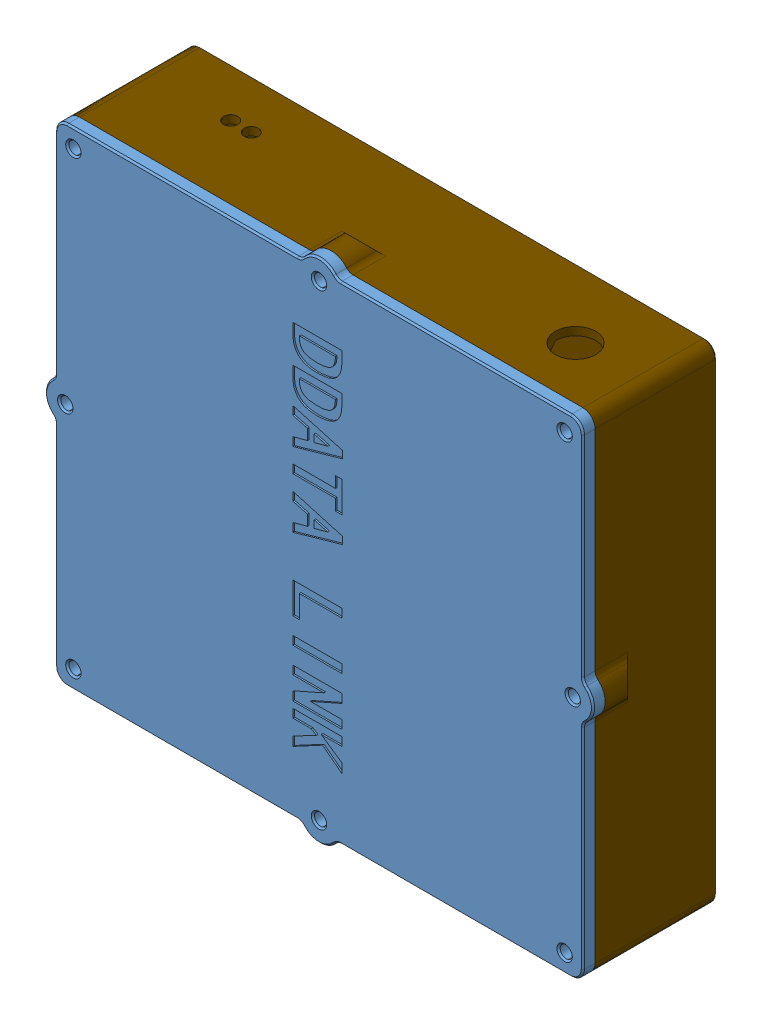
SolidWorks assembly 3D_DATA_LINK_2025-03-18, configuration 默认. Lengths in mm.
Overall size (135 126.5 33).
186 component instances, 20 part files, 8 mates.
Components (placement in the parent):
- 3D_DATA_LINK_2025-03-18.step-1: 3D_DATA_LINK_2025-03-18.step [默认] at (21.7099 -36.6353 -12.5128) size (99.97 88.97 17.5)
  - dtPB-USB5-HDR-TH_P2.54-V-M-R1-C2-S2.54.step-1: dtPB-USB5-HDR-TH_P2.54-V-M-R1-C2-S2.54.step [默认] at (28.7021 69.7231 1.6001) x (0 -1 0) z (0 0 1) size (2.54 5.09 11.5)
    - COMPOUND.step-1: COMPOUND.step [默认] at origin size (2.54 5.09 11.5)
  - dtPB-U3-SOT-23-5_L2.9-W1.6-P0.95-LS2.8-BR.step-1: dtPB-U3-SOT-23-5_L2.9-W1.6-P0.95-LS2.8-BR.step [默认] at (62.6111 64.0081 1.6001) x (-1 0 0) z (0 0 1) size (2.9 2.9 1.1)
    - COMPOUND-0.step-1: COMPOUND-0.step [默认] at origin size (2.9 2.9 1.1)
  - dtPB-I2-CONN-TH_3P-P2.54_2501S-3P.step-1: dtPB-I2-CONN-TH_3P-P2.54_2501S-3P.step [默认] at (107.6962 84.4963 1.6001) x (0 1 0) z (0 0 1) size (10 5.7 10.5)
    - COMPOUND-1.step-1: COMPOUND-1.step [默认] at origin size (10 5.7 10.5)
  - dtPB-I3-CONN-TH_3P-P2.54_2501S-3P.step-1: dtPB-I3-CONN-TH_3P-P2.54_2501S-3P.step [默认] at (100.2607 84.4963 1.6001) x (0 1 0) z (0 0 1) size (10 5.7 10.5)
    - COMPOUND-1.step-1: COMPOUND-1.step [默认] at origin size (10 5.7 10.5)
  - dtPB-I4-CONN-TH_3P-P2.54_2501S-3P.step-1: dtPB-I4-CONN-TH_3P-P2.54_2501S-3P.step [默认] at (92.8252 84.4963 1.6001) x (0 1 0) z (0 0 1) size (10 5.7 10.5)
    - COMPOUND-1.step-1: COMPOUND-1.step [默认] at origin size (10 5.7 10.5)
  - dtPB-I5-CONN-TH_3P-P2.54_2501S-3P.step-1: dtPB-I5-CONN-TH_3P-P2.54_2501S-3P.step [默认] at (85.3896 84.4963 1.6001) x (0 1 0) z (0 0 1) size (10 5.7 10.5)
    - COMPOUND-1.step-1: COMPOUND-1.step [默认] at origin size (10 5.7 10.5)
  - dtPB-I6-CONN-TH_3P-P2.54_2501S-3P.step-1: dtPB-I6-CONN-TH_3P-P2.54_2501S-3P.step [默认] at (63.083 84.4963 1.6001) x (0 1 0) z (0 0 1) size (10 5.7 10.5)
    - COMPOUND-1.step-1: COMPOUND-1.step [默认] at origin size (10 5.7 10.5)
  - dtPB-I7-CONN-TH_3P-P2.54_2501S-3P.step-1: dtPB-I7-CONN-TH_3P-P2.54_2501S-3P.step [默认] at (55.6475 84.4963 1.6001) x (0 1 0) z (0 0 1) size (10 5.7 10.5)
    - COMPOUND-1.step-1: COMPOUND-1.step [默认] at origin size (10 5.7 10.5)
  - dtPB-O1-CONN-TH_3P-P2.54_2501S-3P.step-1: dtPB-O1-CONN-TH_3P-P2.54_2501S-3P.step [默认] at (15.7076 34.7933 1.6001) x (-1 0 0) z (0 0 1) size (10 5.7 10.5)
    - COMPOUND-1.step-1: COMPOUND-1.step [默认] at origin size (10 5.7 10.5)
  - dtPB-O2-CONN-TH_3P-P2.54_2501S-3P.step-1: dtPB-O2-CONN-TH_3P-P2.54_2501S-3P.step [默认] at (15.7076 27.2931 1.6001) x (-1 0 0) z (0 0 1) size (10 5.7 10.5)
    - COMPOUND-1.step-1: COMPOUND-1.step [默认] at origin size (10 5.7 10.5)
  - dtPB-O3-CONN-TH_3P-P2.54_2501S-3P.step-1: dtPB-O3-CONN-TH_3P-P2.54_2501S-3P.step [默认] at (15.621 11.938 1.6001) x (-1 0 0) z (0 0 1) size (10 5.7 10.5)
    - COMPOUND-1.step-1: COMPOUND-1.step [默认] at origin size (10 5.7 10.5)
  - dtPB-O4-CONN-TH_3P-P2.54_2501S-3P.step-1: dtPB-O4-CONN-TH_3P-P2.54_2501S-3P.step [默认] at (15.7076 4.318 1.6001) x (-1 0 0) z (0 0 1) size (10 5.7 10.5)
    - COMPOUND-1.step-1: COMPOUND-1.step [默认] at origin size (10 5.7 10.5)
  - dtPB-O5-CONN-TH_3P-P2.54_2501S-3P.step-1: dtPB-O5-CONN-TH_3P-P2.54_2501S-3P.step [默认] at (26.7971 5.842 1.6001) x (0 -1 0) z (0 0 1) size (10 5.7 10.5)
    - COMPOUND-1.step-1: COMPOUND-1.step [默认] at origin size (10 5.7 10.5)
  - dtPB-O6-CONN-TH_3P-P2.54_2501S-3P.step-1: dtPB-O6-CONN-TH_3P-P2.54_2501S-3P.step [默认] at (34.1313 5.842 1.6001) x (0 -1 0) z (0 0 1) size (10 5.7 10.5)
    - COMPOUND-1.step-1: COMPOUND-1.step [默认] at origin size (10 5.7 10.5)
  - dtPB-O7-CONN-TH_3P-P2.54_2501S-3P.step-1: dtPB-O7-CONN-TH_3P-P2.54_2501S-3P.step [默认] at (41.4656 5.842 1.6001) x (0 -1 0) z (0 0 1) size (10 5.7 10.5)
    - COMPOUND-1.step-1: COMPOUND-1.step [默认] at origin size (10 5.7 10.5)
  - dtPB-PT100-CONN-TH_3P-P2.54_2501S-3P.step-1: dtPB-PT100-CONN-TH_3P-P2.54_2501S-3P.step [默认] at (78.1369 5.842 1.6001) x (0 -1 0) z (0 0 1) size (10 5.7 10.5)
    - COMPOUND-1.step-1: COMPOUND-1.step [默认] at origin size (10 5.7 10.5)
  - dtPB-PT101-CONN-TH_3P-P2.54_2501S-3P.step-1: dtPB-PT101-CONN-TH_3P-P2.54_2501S-3P.step [默认] at (85.4712 5.842 1.6001) x (0 -1 0) z (0 0 1) size (10 5.7 10.5)
    - COMPOUND-1.step-1: COMPOUND-1.step [默认] at origin size (10 5.7 10.5)
  - dtPB-PT102-CONN-TH_3P-P2.54_2501S-3P.step-1: dtPB-PT102-CONN-TH_3P-P2.54_2501S-3P.step [默认] at (105.1963 3.302 1.6001) size (10 5.7 10.5)
    - COMPOUND-1.step-1: COMPOUND-1.step [默认] at origin size (10 5.7 10.5)
  - dtPB-PT103-CONN-TH_3P-P2.54_2501S-3P.step-1: dtPB-PT103-CONN-TH_3P-P2.54_2501S-3P.step [默认] at (105.1963 11.2713 1.6001) size (10 5.7 10.5)
    - COMPOUND-1.step-1: COMPOUND-1.step [默认] at origin size (10 5.7 10.5)
  - dtPB-PWM1-CONN-TH_3P-P2.54_2501S-3P.step-1: dtPB-PWM1-CONN-TH_3P-P2.54_2501S-3P.step [默认] at (15.7076 50.0477 1.6001) x (-1 0 0) z (0 0 1) size (10 5.7 10.5)
    - COMPOUND-1.step-1: COMPOUND-1.step [默认] at origin size (10 5.7 10.5)
  - dtPB-PWM2-CONN-TH_3P-P2.54_2501S-3P.step-1: dtPB-PWM2-CONN-TH_3P-P2.54_2501S-3P.step [默认] at (15.7076 42.4205 1.6001) x (-1 0 0) z (0 0 1) size (10 5.7 10.5)
    - COMPOUND-1.step-1: COMPOUND-1.step [默认] at origin size (10 5.7 10.5)
  - dtPB-PWM3-CONN-TH_3P-P2.54_2501S-3P.step-1: dtPB-PWM3-CONN-TH_3P-P2.54_2501S-3P.step [默认] at (105.1963 59.0869 1.6001) size (10 5.7 10.5)
    - COMPOUND-1.step-1: COMPOUND-1.step [默认] at origin size (10 5.7 10.5)
  - dtPB-PWM4-CONN-TH_3P-P2.54_2501S-3P.step-1: dtPB-PWM4-CONN-TH_3P-P2.54_2501S-3P.step [默认] at (105.1963 67.0561 1.6001) size (10 5.7 10.5)
    - COMPOUND-1.step-1: COMPOUND-1.step [默认] at origin size (10 5.7 10.5)
  - dtPB-PWM5-CONN-TH_3P-P2.54_2501S-3P.step-1: dtPB-PWM5-CONN-TH_3P-P2.54_2501S-3P.step [默认] at (77.9541 84.4963 1.6001) x (0 1 0) z (0 0 1) size (10 5.7 10.5)
    - COMPOUND-1.step-1: COMPOUND-1.step [默认] at origin size (10 5.7 10.5)
  - dtPB-PWM6-CONN-TH_3P-P2.54_2501S-3P.step-1: dtPB-PWM6-CONN-TH_3P-P2.54_2501S-3P.step [默认] at (70.5186 84.4963 1.6001) x (0 1 0) z (0 0 1) size (10 5.7 10.5)
    - COMPOUND-1.step-1: COMPOUND-1.step [默认] at origin size (10 5.7 10.5)
  - dtPB-CURRENT1-CONN-TH_3P-P2.54_2501S-3P.step-1: dtPB-CURRENT1-CONN-TH_3P-P2.54_2501S-3P.step [默认] at (63.4684 5.842 1.6001) x (0 -1 0) z (0 0 1) size (10 5.7 10.5)
    - COMPOUND-1.step-1: COMPOUND-1.step [默认] at origin size (10 5.7 10.5)
  - dtPB-CURRENT2-CONN-TH_3P-P2.54_2501S-3P.step-1: dtPB-CURRENT2-CONN-TH_3P-P2.54_2501S-3P.step [默认] at (70.8026 5.842 1.6001) x (0 -1 0) z (0 0 1) size (10 5.7 10.5)
    - COMPOUND-1.step-1: COMPOUND-1.step [默认] at origin size (10 5.7 10.5)
  - dtPB-CURRENT3-CONN-TH_3P-P2.54_2501S-3P.step-1: dtPB-CURRENT3-CONN-TH_3P-P2.54_2501S-3P.step [默认] at (105.1963 19.2405 1.6001) size (10 5.7 10.5)
    - COMPOUND-1.step-1: COMPOUND-1.step [默认] at origin size (10 5.7 10.5)
  - dtPB-CURRENT4-CONN-TH_3P-P2.54_2501S-3P.step-1: dtPB-CURRENT4-CONN-TH_3P-P2.54_2501S-3P.step [默认] at (105.1963 27.2098 1.6001) size (10 5.7 10.5)
    - COMPOUND-1.step-1: COMPOUND-1.step [默认] at origin size (10 5.7 10.5)
  - dtPB-FLOW1-CONN-TH_3P-P2.54_2501S-3P.step-1: dtPB-FLOW1-CONN-TH_3P-P2.54_2501S-3P.step [默认] at (105.1963 35.1791 1.6001) size (10 5.7 10.5)
    - COMPOUND-1.step-1: COMPOUND-1.step [默认] at origin size (10 5.7 10.5)
  - dtPB-FLOW2-CONN-TH_3P-P2.54_2501S-3P.step-1: dtPB-FLOW2-CONN-TH_3P-P2.54_2501S-3P.step [默认] at (105.1963 43.1483 1.6001) size (10 5.7 10.5)
    - COMPOUND-1.step-1: COMPOUND-1.step [默认] at origin size (10 5.7 10.5)
  - dtPB-FLOW3-CONN-TH_3P-P2.54_2501S-3P.step-1: dtPB-FLOW3-CONN-TH_3P-P2.54_2501S-3P.step [默认] at (48.7998 5.842 1.6001) x (0 -1 0) z (0 0 1) size (10 5.7 10.5)
    - COMPOUND-1.step-1: COMPOUND-1.step [默认] at origin size (10 5.7 10.5)
  - dtPB-FLOW4-CONN-TH_3P-P2.54_2501S-3P.step-1: dtPB-FLOW4-CONN-TH_3P-P2.54_2501S-3P.step [默认] at (56.1341 5.842 1.6001) x (0 -1 0) z (0 0 1) size (10 5.7 10.5)
    - COMPOUND-1.step-1: COMPOUND-1.step [默认] at origin size (10 5.7 10.5)
  - dtPB-I1-CONN-TH_3P-P2.54_2501S-3P.step-1: dtPB-I1-CONN-TH_3P-P2.54_2501S-3P.step [默认] at (105.1963 51.1176 1.6001) size (10 5.7 10.5)
    - COMPOUND-1.step-1: COMPOUND-1.step [默认] at origin size (10 5.7 10.5)
  - dtPB-R2-R0603.step-1: dtPB-R2-R0603.step [默认] at (41.0617 61.009 1.6001) x (0 1 0) z (0 0 1) size (1.62 0.81 0.45)
    - COMPOUND-2.step-1: COMPOUND-2.step [默认] at origin size (1.62 0.81 0.45)
  - dtPB-R3-R0603.step-1: dtPB-R3-R0603.step [默认] at (41.0211 57.4041 1.6001) x (0 1 0) z (0 0 1) size (1.62 0.81 0.45)
    - COMPOUND-2.step-1: COMPOUND-2.step [默认] at origin size (1.62 0.81 0.45)
  - dtPB-R4-R0603.step-1: dtPB-R4-R0603.step [默认] at (40.0051 53.5941 1.6001) x (-1 0 0) z (0 0 1) size (1.62 0.81 0.45)
    - COMPOUND-2.step-1: COMPOUND-2.step [默认] at origin size (1.62 0.81 0.45)
  - dtPB-R5-R0603.step-1: dtPB-R5-R0603.step [默认] at (36.7031 53.5941 1.6001) x (-1 0 0) z (0 0 1) size (1.62 0.81 0.45)
    - COMPOUND-2.step-1: COMPOUND-2.step [默认] at origin size (1.62 0.81 0.45)
  - dtPB-R6-R0603.step-1: dtPB-R6-R0603.step [默认] at (60.8331 29.3371 1.6001) x (0 1 0) z (0 0 1) size (1.62 0.81 0.45)
    - COMPOUND-2.step-1: COMPOUND-2.step [默认] at origin size (1.62 0.81 0.45)
  - dtPB-R7-R0603.step-1: dtPB-R7-R0603.step [默认] at (33.1471 71.5011 1.6001) size (1.62 0.81 0.45)
    - COMPOUND-2.step-1: COMPOUND-2.step [默认] at origin size (1.62 0.81 0.45)
  - dtPB-R8-R0603.step-1: dtPB-R8-R0603.step [默认] at (58.5471 39.6241 1.6001) x (-1 0 0) z (0 0 1) size (1.62 0.81 0.45)
    - COMPOUND-2.step-1: COMPOUND-2.step [默认] at origin size (1.62 0.81 0.45)
  - dtPB-R9-R0603.step-1: dtPB-R9-R0603.step [默认] at (69.5961 29.5911 1.6001) x (0 1 0) z (0 0 1) size (1.62 0.81 0.45)
    - COMPOUND-2.step-1: COMPOUND-2.step [默认] at origin size (1.62 0.81 0.45)
  - dtPB-R18-R0603.step-1: dtPB-R18-R0603.step [默认] at (98.9529 37.3381 1.6001) x (0 -1 0) z (0 0 1) size (1.62 0.81 0.45)
    - COMPOUND-2.step-1: COMPOUND-2.step [默认] at origin size (1.62 0.81 0.45)
  - dtPB-R19-R0603.step-1: dtPB-R19-R0603.step [默认] at (98.9529 45.3724 1.6001) x (0 -1 0) z (0 0 1) size (1.62 0.81 0.45)
    - COMPOUND-2.step-1: COMPOUND-2.step [默认] at origin size (1.62 0.81 0.45)
  - dtPB-R20-R0603.step-1: dtPB-R20-R0603.step [默认] at (51.0541 12.3458 1.6001) x (-1 0 0) z (0 0 1) size (1.62 0.81 0.45)
    - COMPOUND-2.step-1: COMPOUND-2.step [默认] at origin size (1.62 0.81 0.45)
  - dtPB-R21-R0603.step-1: dtPB-R21-R0603.step [默认] at (58.4508 12.4728 1.6001) x (-1 0 0) z (0 0 1) size (1.62 0.81 0.45)
    - COMPOUND-2.step-1: COMPOUND-2.step [默认] at origin size (1.62 0.81 0.45)
  - dtPB-R22-R0603.step-1: dtPB-R22-R0603.step [默认] at (62.2301 12.4728 1.6001) size (1.62 0.81 0.45)
    - COMPOUND-2.step-1: COMPOUND-2.step [默认] at origin size (1.62 0.81 0.45)
  - dtPB-R23-R0603.step-1: dtPB-R23-R0603.step [默认] at (69.5961 12.3458 1.6001) size (1.62 0.81 0.45)
    - COMPOUND-2.step-1: COMPOUND-2.step [默认] at origin size (1.62 0.81 0.45)
  - dtPB-R24-R0603.step-1: dtPB-R24-R0603.step [默认] at (98.8062 18.161 1.6001) x (0 1 0) z (0 0 1) size (1.62 0.81 0.45)
    - COMPOUND-2.step-1: COMPOUND-2.step [默认] at origin size (1.62 0.81 0.45)
  - dtPB-R25-R0603.step-1: dtPB-R25-R0603.step [默认] at (98.8259 25.7811 1.6001) x (0 1 0) z (0 0 1) size (1.62 0.81 0.45)
    - COMPOUND-2.step-1: COMPOUND-2.step [默认] at origin size (1.62 0.81 0.45)
  - dtPB-R26-R0603.step-1: dtPB-R26-R0603.step [默认] at (76.8969 12.4217 1.6001) size (1.62 0.81 0.45)
    - COMPOUND-2.step-1: COMPOUND-2.step [默认] at origin size (1.62 0.81 0.45)
  - dtPB-R27-R0603.step-1: dtPB-R27-R0603.step [默认] at (80.3912 12.446 1.6001) x (-1 0 0) z (0 0 1) size (1.62 0.81 0.45)
    - COMPOUND-2.step-1: COMPOUND-2.step [默认] at origin size (1.62 0.81 0.45)
  - dtPB-R28-R0603.step-1: dtPB-R28-R0603.step [默认] at (97.9172 2.54 1.6001) x (0 1 0) z (0 0 1) size (1.62 0.81 0.45)
    - COMPOUND-2.step-1: COMPOUND-2.step [默认] at origin size (1.62 0.81 0.45)
  - dtPB-R29-R0603.step-1: dtPB-R29-R0603.step [默认] at (97.9172 5.969 1.6001) x (0 -1 0) z (0 0 1) size (1.62 0.81 0.45)
    - COMPOUND-2.step-1: COMPOUND-2.step [默认] at origin size (1.62 0.81 0.45)
  - dtPB-R30-R0603.step-1: dtPB-R30-R0603.step [默认] at (97.9172 10.16 1.6001) x (0 1 0) z (0 0 1) size (1.62 0.81 0.45)
    - COMPOUND-2.step-1: COMPOUND-2.step [默认] at origin size (1.62 0.81 0.45)
  - dtPB-R31-R0603.step-1: dtPB-R31-R0603.step [默认] at (97.9725 13.4275 1.6001) x (0 -1 0) z (0 0 1) size (1.62 0.81 0.45)
    - COMPOUND-2.step-1: COMPOUND-2.step [默认] at origin size (1.62 0.81 0.45)
  - dtPB-R32-R0603.step-1: dtPB-R32-R0603.step [默认] at (84.2565 12.4217 1.6001) size (1.62 0.81 0.45)
    - COMPOUND-2.step-1: COMPOUND-2.step [默认] at origin size (1.62 0.81 0.45)
  - dtPB-R33-R0603.step-1: dtPB-R33-R0603.step [默认] at (87.6855 12.4217 1.6001) x (-1 0 0) z (0 0 1) size (1.62 0.81 0.45)
    - COMPOUND-2.step-1: COMPOUND-2.step [默认] at origin size (1.62 0.81 0.45)
  - dtPB-R1-R0603.step-1: dtPB-R1-R0603.step [默认] at (41.0211 64.5161 1.6001) x (0 1 0) z (0 0 1) size (1.62 0.81 0.45)
    - COMPOUND-2.step-1: COMPOUND-2.step [默认] at origin size (1.62 0.81 0.45)
  - dtPB-IC1-CONN-TH_4P-P2.50_4PIN.step-1: dtPB-IC1-CONN-TH_4P-P2.50_4PIN.step [默认] at (16.891 19.558 1.6001) x (-1 0 0) z (0 0 1) size (12.5 5.7 10)
    - COMPOUND-3.step-1: COMPOUND-3.step [默认] at origin size (12.5 5.7 10)
  - dtPB-USART1-CONN-TH_4P-P2.50_4PIN.step-1: dtPB-USART1-CONN-TH_4P-P2.50_4PIN.step [默认] at (48.0061 83.2532 1.6001) x (0 1 0) z (0 0 1) size (12.5 5.7 10)
    - COMPOUND-3.step-1: COMPOUND-3.step [默认] at origin size (12.5 5.7 10)
  - dtPB-DOWNLOAD1-CONN-TH_4P-P2.50_4PIN.step-1: dtPB-DOWNLOAD1-CONN-TH_4P-P2.50_4PIN.step [默认] at (16.891 57.9121 1.6001) x (-1 0 0) z (0 0 1) size (12.5 5.7 10)
    - COMPOUND-3.step-1: COMPOUND-3.step [默认] at origin size (12.5 5.7 10)
  - dtPB-U5-WIRELM-SMD_E43-433T13S3.step-1: dtPB-U5-WIRELM-SMD_E43-433T13S3.step [默认] at (35.0521 31.2421 1.6001) x (-1 0 0) z (0 0 1) size (16 26 3.23)
    - COMPOUND-4.step-1: COMPOUND-4.step [默认] at origin size (16 26 3.23)
  - dtPB-VCC1-CONN-TH_2P-P5.00_WJ500V-5.08-2P.step-1: dtPB-VCC1-CONN-TH_2P-P5.00_WJ500V-5.08-2P.step [默认] at (20.32 83.8202 1.6001) size (10.76 10 17.5)
    - COMPOUND-5.step-1: COMPOUND-5.step [默认] at origin size (10.76 10 17.5)
  - dtPB-V5-CONN-TH_2P-P2.50_HX25003-2A.step-1: dtPB-V5-CONN-TH_2P-P2.50_HX25003-2A.step [默认] at (14.351 66.0401 1.6001) size (7.5 5.9 10.6)
    - COMPOUND-6.step-1: COMPOUND-6.step [默认] at origin size (7.5 5.9 10.6)
  - dtPB-U2-SOT-23-6_L2.9-W1.6-P0.95-LS2.8-BL.step-1: dtPB-U2-SOT-23-6_L2.9-W1.6-P0.95-LS2.8-BL.step [默认] at (36.4491 56.7691 1.6001) x (0 -1 0) z (0 0 1) size (2.88 2.79 1.64)
    - COMPOUND-7.step-1: COMPOUND-7.step [默认] at origin size (2.88 2.79 1.64)
  - dtPB-U1-LQFP-64_L10.0-W10.0-P0.50-LS12.0-BL.step-1: dtPB-U1-LQFP-64_L10.0-W10.0-P0.50-LS12.0-BL.step [默认] at (70.3581 41.6561 1.6001) size (12 12 1.45)
    - COMPOUND-8.step-1: COMPOUND-8.step [默认] at origin size (12 12 1.45)
  - dtPB-Board.step-1: dtPB-Board.step [默认] at origin size (99.97 88.97 1.6)
  - dtPB-C137-CAP-SMD_BD6.3-L6.6-W6.6-LS7.6-FD-1.step-1: dtPB-C137-CAP-SMD_BD6.3-L6.6-W6.6-LS7.6-FD-1.step [默认] at (20.447 73.1521 1.6001) size (7.2 6.6 7.72)
  - dtPB-C137-CAP-SMD_BD6.3-L6.6-W6.6-LS7.6-FD-1.step-2: dtPB-C137-CAP-SMD_BD6.3-L6.6-W6.6-LS7.6-FD-1.step [默认] at (49.9111 60.8331 1.6001) x (0 -1 0) z (0 0 1) size (7.2 6.6 7.72)
  - dtPB-C1-C0805.step-1: dtPB-C1-C0805.step [默认] at (35.9411 64.0081 1.6001) x (0 1 0) z (0 0 1) size (2 1.3 1.3)
  - dtPB-C1-C0805.step-2: dtPB-C1-C0805.step [默认] at (38.4811 64.0081 1.6001) x (0 1 0) z (0 0 1) size (2 1.3 1.3)
  - dtPB-C1-C0805.step-3: dtPB-C1-C0805.step [默认] at (49.5301 42.5451 1.6001) x (0 -1 0) z (0 0 1) size (2 1.3 1.3)
  - dtPB-C1-C0805.step-4: dtPB-C1-C0805.step [默认] at (30.3531 55.3721 1.6001) x (0 -1 0) z (0 0 1) size (2 1.3 1.3)
  - dtPB-C2-C0603.step-1: dtPB-C2-C0603.step [默认] at (43.1801 60.9601 1.6001) x (0 1 0) z (0 0 1) size (1.6 0.8 0.8)
  - dtPB-C2-C0603.step-2: dtPB-C2-C0603.step [默认] at (36.1951 60.1981 1.6001) x (-1 0 0) z (0 0 1) size (1.6 0.8 0.8)
  - dtPB-C2-C0603.step-3: dtPB-C2-C0603.step [默认] at (59.0551 64.2621 1.6001) x (0 1 0) z (0 0 1) size (1.6 0.8 0.8)
  - dtPB-C2-C0603.step-4: dtPB-C2-C0603.step [默认] at (65.9131 64.1351 1.6001) x (0 1 0) z (0 0 1) size (1.6 0.8 0.8)
  - dtPB-C2-C0603.step-5: dtPB-C2-C0603.step [默认] at (58.5471 37.5921 1.6001) size (1.6 0.8 0.8)
  - dtPB-C2-C0603.step-6: dtPB-C2-C0603.step [默认] at (73.716 29.5848 1.6001) x (0 1 0) z (0 0 1) size (1.6 0.8 0.8)
  - dtPB-C2-C0603.step-7: dtPB-C2-C0603.step [默认] at (84.5822 38.8621 1.6001) size (1.6 0.8 0.8)
  - dtPB-C2-C0603.step-8: dtPB-C2-C0603.step [默认] at (66.5481 55.2451 1.6001) x (0 -1 0) z (0 0 1) size (1.6 0.8 0.8)
  - dtPB-C2-C0603.step-9: dtPB-C2-C0603.step [默认] at (84.5822 45.7201 1.6001) size (1.6 0.8 0.8)
  - dtPB-C2-C0603.step-10: dtPB-C2-C0603.step [默认] at (63.8896 25.3945 1.6001) x (0 1 0) z (0 0 1) size (1.6 0.8 0.8)
  - dtPB-C2-C0603.step-11: dtPB-C2-C0603.step [默认] at (66.1671 25.4001 1.6001) x (0 1 0) z (0 0 1) size (1.6 0.8 0.8)
  - dtPB-C2-C0603.step-12: dtPB-C2-C0603.step [默认] at (71.3741 29.5911 1.6001) x (0 -1 0) z (0 0 1) size (1.6 0.8 0.8)
  - dtPB-C2-C0603.step-13: dtPB-C2-C0603.step [默认] at (46.7361 42.0371 1.6001) x (0 -1 0) z (0 0 1) size (1.6 0.8 0.8)
  - dtPB-C2-C0603.step-14: dtPB-C2-C0603.step [默认] at (77.0231 14.8655 1.6001) size (1.6 0.8 0.8)
  - dtPB-C2-C0603.step-15: dtPB-C2-C0603.step [默认] at (80.4521 14.8655 1.6001) size (1.6 0.8 0.8)
  - dtPB-C2-C0603.step-16: dtPB-C2-C0603.step [默认] at (84.2626 14.8655 1.6001) size (1.6 0.8 0.8)
  - dtPB-C2-C0603.step-17: dtPB-C2-C0603.step [默认] at (87.6938 14.8655 1.6001) size (1.6 0.8 0.8)
  - dtPB-C2-C0603.step-18: dtPB-C2-C0603.step [默认] at (95.7582 2.54 1.6001) x (0 1 0) z (0 0 1) size (1.6 0.8 0.8)
  - dtPB-C2-C0603.step-19: dtPB-C2-C0603.step [默认] at (95.7582 5.969 1.6001) x (0 1 0) z (0 0 1) size (1.6 0.8 0.8)
  - dtPB-C2-C0603.step-20: dtPB-C2-C0603.step [默认] at (95.7582 13.462 1.6001) x (0 1 0) z (0 0 1) size (1.6 0.8 0.8)
  - dtPB-C2-C0603.step-21: dtPB-C2-C0603.step [默认] at (95.7582 10.16 1.6001) x (0 1 0) z (0 0 1) size (1.6 0.8 0.8)
  - dtPB-C2-C0603.step-22: dtPB-C2-C0603.step [默认] at (98.9796 33.9424 1.6001) x (0 1 0) z (0 0 1) size (1.6 0.8 0.8)
  - dtPB-C2-C0603.step-23: dtPB-C2-C0603.step [默认] at (98.9796 42.1974 1.6001) x (0 1 0) z (0 0 1) size (1.6 0.8 0.8)
  - dtPB-C2-C0603.step-24: dtPB-C2-C0603.step [默认] at (55.1055 12.446 1.6001) size (1.6 0.8 0.8)
  - dtPB-C2-C0603.step-25: dtPB-C2-C0603.step [默认] at (47.6251 12.446 1.6001) size (1.6 0.8 0.8)
  - dtPB-C2-C0603.step-26: dtPB-C2-C0603.step [默认] at (73.1521 12.4514 1.6001) x (-1 0 0) z (0 0 1) size (1.6 0.8 0.8)
  - dtPB-C2-C0603.step-27: dtPB-C2-C0603.step [默认] at (98.8472 29.2773 1.6001) x (0 -1 0) z (0 0 1) size (1.6 0.8 0.8)
  - dtPB-C2-C0603.step-28: dtPB-C2-C0603.step [默认] at (98.8472 21.463 1.6001) x (0 -1 0) z (0 0 1) size (1.6 0.8 0.8)
  - dtPB-C2-C0603.step-29: dtPB-C2-C0603.step [默认] at (65.7861 12.4514 1.6001) x (-1 0 0) z (0 0 1) size (1.6 0.8 0.8)
  - dtPB-C2-C0603.step-30: dtPB-C2-C0603.step [默认] at (98.4252 52.7051 1.6001) x (0 -1 0) z (0 0 1) size (1.6 0.8 0.8)
  - dtPB-C2-C0603.step-31: dtPB-C2-C0603.step [默认] at (83.9472 77.4702 1.6001) size (1.6 0.8 0.8)
  - dtPB-C2-C0603.step-32: dtPB-C2-C0603.step [默认] at (105.9594 77.4702 1.6001) size (1.6 0.8 0.8)
  - dtPB-C2-C0603.step-33: dtPB-C2-C0603.step [默认] at (61.4681 77.4702 1.6001) size (1.6 0.8 0.8)
  - dtPB-C2-C0603.step-34: dtPB-C2-C0603.step [默认] at (91.1862 77.4702 1.6001) size (1.6 0.8 0.8)
  - dtPB-C2-C0603.step-35: dtPB-C2-C0603.step [默认] at (54.2997 77.4702 1.6001) size (1.6 0.8 0.8)
  - dtPB-C2-C0603.step-36: dtPB-C2-C0603.step [默认] at (98.8062 77.4702 1.6001) size (1.6 0.8 0.8)
  - dtPB-C2-C0603.step-37: dtPB-C2-C0603.step [默认] at (58.4201 35.4331 1.6001) size (1.6 0.8 0.8)
  - dtPB-C2-C0603.step-38: dtPB-C2-C0603.step [默认] at (32.7661 55.8801 1.6001) x (0 -1 0) z (0 0 1) size (1.6 0.8 0.8)
  - dtPB-L1-IND-SMD_L7.3-W6.8.step-1: dtPB-L1-IND-SMD_L7.3-W6.8.step [默认] at (30.3531 62.4841 1.6001) x (0 1 0) z (0 0 1) size (7.42 6.8 3.05)
  - dtPB-X1-OSC-SMD_4P-L3.2-W2.5-BL.step-1: dtPB-X1-OSC-SMD_4P-L3.2-W2.5-BL.step [默认] at (64.8971 29.3371 1.6001) size (3.2 2.5 0.81)
  - dtPB-USB1-USB-B_TH_BF90.step-1: dtPB-USB1-USB-B_TH_BF90.step [默认] at (34.0361 76.9622 1.6001) x (-1 0 0) z (0 0 1) size (14.04 16.2 13.8)
- data_link_盒子-1: data_link_盒子 [默认] at (17.1401 68.4648 -19.5128) x (0 -1 0) z (-1 0 0) size (125 30 135)
- data_link_盒子_盖子-1: data_link_盒子_盖子 [默认] at (17.1401 -51.5352 13.4872) x (0 1 0) z (-1 0 0) size (125 3 135)
- sma座-1: sma座 [默认] at (116.1401 -49.5352 -3.5128) x (-0.514329 0 -0.857593) z (-0.857593 0 0.514329) size (10 36 10)
Mates (geometry in assembly coordinates):
- 重合4: coincident anti-aligned: plane of data_link_盒子-1 through (17.1401 68.4648 10.4872) normal (0 0 1); plane of data_link_盒子_盖子-1 through (17.1401 -51.5352 10.4872) normal (0 0 -1)
- 同心5: concentric aligned: cylinder of data_link_盒子-1 through (116.1401 -59.5352 -3.5128) axis (0 1 0) radius 3.25; cylinder of sma座-1 through (116.1401 -55.5352 -3.5128) axis (0 1 0) radius 3.175
- 重合5: coincident anti-aligned: plane of data_link_盒子-1 through (19.1401 -49.5352 10.4872) normal (0 1 0); plane of sma座-1 through (116.1401 -49.5352 -3.5128) normal (0 -1 0)
- 重合6: coincident anti-aligned: plane of 3D_DATA_LINK_2025-03-18.step-1/dtPB-Board.step-1 through (82.124 8.5268 -12.5128) normal (0 0 -1); plane of data_link_盒子-1 through (116.7101 25.3648 -12.5128) normal (0 0 1)
- 同心6: concentric anti-aligned: cylinder of 3D_DATA_LINK_2025-03-18.step-1/dtPB-Board.step-1 through (116.7101 25.3648 -12.5128) axis (0 0 -1) radius 1.6; circle of data_link_盒子-1
- 平行1: parallel: line of 3D_DATA_LINK_2025-03-18.step-1/dtPB-Board.step-1 through (32.1366 53.0141 -10.9127) axis (1 0 0); plane of data_link_盒子-1 through (17.1401 68.4648 -17.5128) normal (0 1 0)
- 同心7: concentric aligned: circle of data_link_盒子-1; cylinder of data_link_盒子_盖子-1 through (144.6401 8.4648 10.4872) axis (0 0 1) radius 1.5
- 同心10: concentric aligned: cylinder of data_link_盒子-1 through (19.6401 8.4648 5.4872) axis (0 0 1) radius 1.4; cylinder of data_link_盒子_盖子-1 through (19.6401 8.4648 10.4872) axis (0 0 1) radius 1.5
